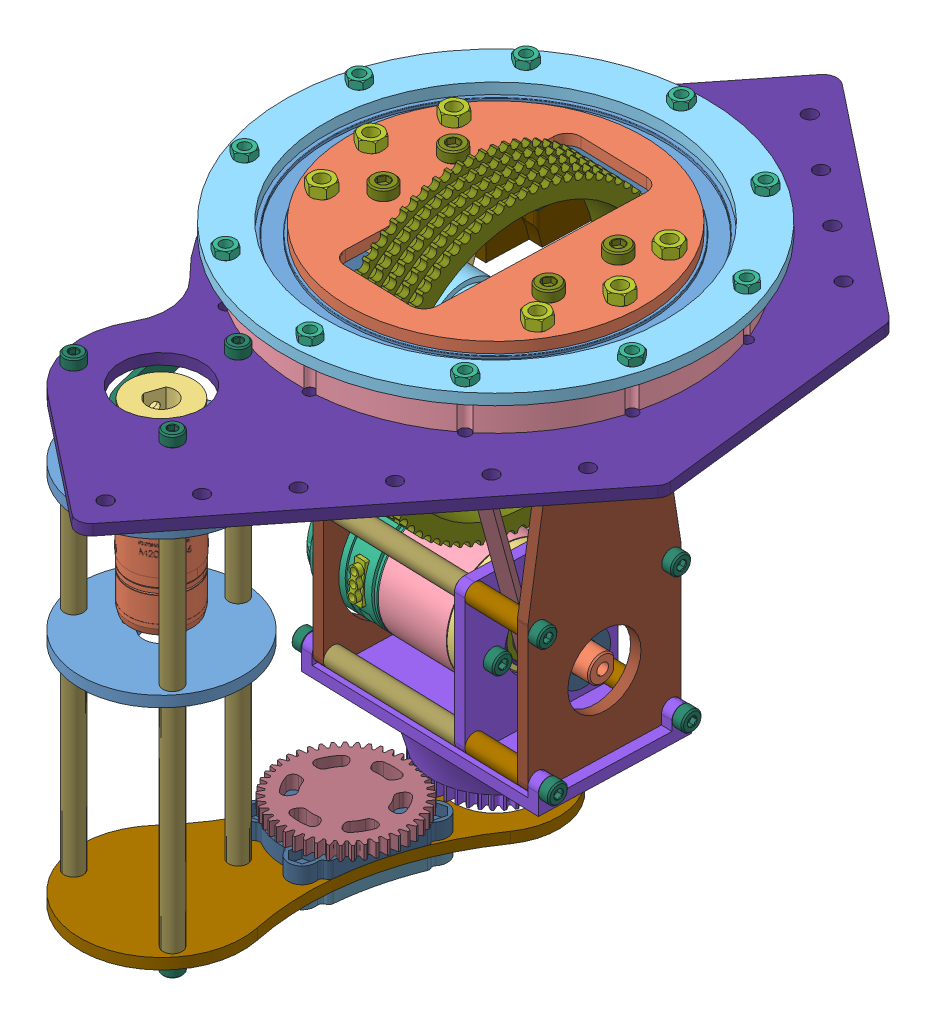
SolidWorks assembly 舵轮装配, configuration 默认. Lengths in mm. (continued)
Mates (geometry in assembly coordinates): (continued)
- 同心68: concentric aligned: cylinder of M3508电机安装延长-1 through (8.8031 -96.0384 93.3761) axis (-0.999547 0 -0.03008) radius 2.1; cylinder of M4螺丝头-14 through (12.8013 -96.0384 93.4965) axis (-0.999547 0 -0.03008) radius 3.6
- 同心69: concentric aligned: cylinder of M3508电机安装延长-1 through (9.3295 -113.5384 75.8841) axis (-0.999547 0 -0.03008) radius 2.1; cylinder of M4螺丝头-13 through (13.3277 -113.5384 76.0044) axis (-0.999547 0 -0.03008) radius 3.6
- 重合43: coincident anti-aligned: plane of M3508电机安装延长-1 through (8.8031 -113.5384 93.3761) normal (0.999547 0 0.03008); plane of M4螺丝头-11 through (8.2767 -113.5384 110.8682) normal (-0.999547 0 -0.03008)
- 重合44: coincident aligned: plane of M4螺丝头-11 through (12.2749 -113.5384 110.9885) normal (0.999547 0 0.03008); plane of M4螺丝头-14 through (12.8013 -96.0384 93.4965) normal (0.999547 0 0.03008)
- 重合45: coincident aligned: plane of M4螺丝头-12 through (12.8013 -131.0384 93.4965) normal (0.999547 0 0.03008); circle of M4螺丝头-13
- 重合46: coincident aligned: plane of M4螺丝头-11 through (12.2749 -113.5384 110.9885) normal (0.999547 0 0.03008); plane of M4螺丝头-12 through (12.8013 -131.0384 93.4965) normal (0.999547 0 0.03008)
- 同心70: concentric anti-aligned: cylinder of M3508电机安装板B-1 through (-45.4733 -15.0564 101.7473) axis (-0.999547 0 -0.03008) radius 2.6; cylinder of M5螺丝头-3 through (-54.4692 -15.0564 101.4766) axis (0.999547 0 0.03008) radius 4.35
- 同心71: concentric anti-aligned: cylinder of M3508电机安装板B-1 through (-44.8717 -15.0564 81.7563) axis (-0.999547 0 -0.03008) radius 2.6; cylinder of M5螺丝头-4 through (-53.8676 -15.0564 81.4856) axis (0.999547 0 0.03008) radius 4.35
- 重合47: coincident anti-aligned: plane of M3508电机安装板B-1 through (-49.1707 -7.5564 91.6315) normal (-0.999547 0 -0.03008); circle of M5螺丝头-4
- 重合48: coincident anti-aligned: plane of M3508电机安装板B-1 through (-49.1707 -7.5564 91.6315) normal (-0.999547 0 -0.03008); plane of M5螺丝头-3 through (-49.4715 -15.0564 101.627) normal (0.999547 0 0.03008)
- 同心72: concentric anti-aligned: cylinder of M3508电机安装板B-1 through (-45.3229 -0.0564 96.7496) axis (-0.999547 0 -0.03008) radius 2.6; cylinder of M5螺丝头-2 through (-54.3188 -0.0564 96.4788) axis (0.999547 0 0.03008) radius 4.35
- 重合49: coincident anti-aligned: plane of M3508电机安装板B-1 through (-49.1707 -7.5564 91.6315) normal (-0.999547 0 -0.03008); plane of M5螺丝头-2 through (-49.3211 -0.0564 96.6292) normal (0.999547 0 0.03008)
- 重合50: coincident anti-aligned: plane of M3508电机安装板B-1 through (-49.1707 -7.5564 91.6315) normal (-0.999547 0 -0.03008); plane of M5螺丝头-1 through (-49.0203 -0.0564 86.6338) normal (0.999547 0 0.03008)
- 同心73: concentric anti-aligned: cylinder of M3508电机安装板B-1 through (-45.0221 -0.0564 86.7541) axis (-0.999547 0 -0.03008) radius 2.6; cylinder of M5螺丝头-1 through (-54.018 -0.0564 86.4834) axis (0.999547 0 0.03008) radius 4.35
- 同心78: concentric aligned: cylinder of HRB 61821薄圈轴承-1 through (-8.689 4.9436 92.8497) axis (0 -1 0) radius 65; cylinder of 舵轮直角安装架-1 through (-8.689 -8.0564 92.8497) axis (0 -1 0) radius 63
- 重合56: coincident anti-aligned: plane of 舵轮上底板-1 through (-8.689 -12.0564 92.8497) normal (0 -1 0); plane of 舵轮转向同步轮 75齿-3 through (-8.6606 -12.0564 92.6837) normal (0 1 0)
- 同心92: concentric aligned: cylinder of 舵轮上底板-1 through (31.7142 -2.0564 117.8264) axis (0 -1 0) radius 2.6; cylinder of 舵轮轴承契合垫B-1 through (31.7142 4.9436 117.8264) axis (0 -1 0) radius 2.6
- 同心93: concentric aligned: cylinder of 舵轮上底板-1 through (31.7142 -2.0564 117.8264) axis (0 -1 0) radius 2.6; cylinder of 舵轮转向同步轮 75齿-3 through (31.7142 23.4436 117.8264) axis (0 -1 0) radius 2.6
- 同心94: concentric aligned: cylinder of 舵轮上底板-1 through (-49.0922 -2.0564 67.8731) axis (0 -1 0) radius 2.6; cylinder of 舵轮转向同步轮 75齿-3 through (-49.0922 23.4436 67.8731) axis (0 -1 0) radius 2.6
- 同心95: concentric aligned: cylinder of 舵轮直角安装架-1 through (-15.1983 -18.0564 205.8519) axis (0 1 0) radius 2.1; cylinder of 舵轮转向电机安装件-1 through (-15.1983 -36.0564 205.8519) axis (0 1 0) radius 2.1
- 同心98: concentric aligned: cylinder of 舵轮直角安装架-1 through (-15.1983 -18.0564 205.8519) axis (0 1 0) radius 2.1; cylinder of 舵轮转向电机安装件-1 through (-15.1983 -36.0564 205.8519) axis (0 1 0) radius 2.1
- 同心99: concentric aligned: cylinder of 舵轮直角安装架-1 through (-58.0411 -18.0564 199.5679) axis (0 1 0) radius 2.1; cylinder of 舵轮转向电机安装件-1 through (-58.0411 -36.0564 199.5679) axis (0 1 0) radius 2.1
- 同心100: concentric aligned: cylinder of 舵轮转向电机安装件-1 through (-33.427 -49.0564 180.9428) axis (0 1 0) radius 1.6; cylinder of RoboMaster M2006 P36直流无刷减速电机.step-2 through (-33.427 -36.0564 180.9428) axis (0 1 0) radius 1.25
- 重合57: coincident anti-aligned: plane of 舵轮转向电机安装件-1 through (-34.8056 -36.0564 190.3422) normal (0 -1 0); plane of RoboMaster M2006 P36直流无刷减速电机.step-2 through (-25.2372 -36.0564 197.911) normal (0 1 0)
- 同心101: concentric aligned: cylinder of 舵轮转向电机安装件-1 through (-34.8056 -49.0564 190.3422) axis (0 1 0) radius 6.6; cylinder of RoboMaster M2006 P36直流无刷减速电机.step-2 through (-34.8056 -19.0564 190.3422) axis (0 1 0) radius 3
- 同心102: concentric anti-aligned: cylinder of 舵轮直角安装架-1 through (-58.0411 -18.0564 199.5679) axis (0 1 0) radius 2.1; cylinder of 螺纹M4_长度20铝柱-5 through (-58.0411 -12.0564 199.5679) axis (0 -1 0) radius 3.5
- 同心103: concentric anti-aligned: cylinder of 舵轮直角安装架-1 through (-31.1775 -18.0564 165.6069) axis (0 1 0) radius 2.1; cylinder of 螺纹M4_长度20铝柱-7 through (-31.1775 -12.0564 165.6069) axis (0 -1 0) radius 3.5
- 同心104: concentric anti-aligned: cylinder of 舵轮直角安装架-1 through (-15.1983 -18.0564 205.8519) axis (0 1 0) radius 2.1; cylinder of 螺纹M4_长度20铝柱-6 through (-15.1983 -12.0564 205.8519) axis (0 -1 0) radius 3.5
- 重合58: coincident anti-aligned: plane of 舵轮转向电机安装件-1 through (-34.8056 -32.0564 190.3422) normal (0 1 0); plane of 螺纹M4_长度20铝柱-6 through (-15.1983 -32.0564 205.8519) normal (0 -1 0)
- 重合59: coincident anti-aligned: plane of 舵轮转向电机安装件-1 through (-34.8056 -32.0564 190.3422) normal (0 1 0); plane of 螺纹M4_长度20铝柱-5 through (-58.0411 -32.0564 199.5679) normal (0 -1 0)
- 重合60: coincident anti-aligned: plane of 舵轮转向电机安装件-1 through (-34.8056 -32.0564 190.3422) normal (0 1 0); plane of 螺纹M4_长度20铝柱-7 through (-31.1775 -32.0564 165.6069) normal (0 -1 0)
- 重合61: coincident anti-aligned: plane of 舵轮直角安装架-1 through (-8.689 -12.0564 92.8497) normal (0 -1 0); plane of 螺纹M4_长度20铝柱-5 through (-58.0411 -12.0564 199.5679) normal (0 1 0)
- 同心105: concentric anti-aligned: cylinder of RoboMaster M2006 P36直流无刷减速电机.step-2 through (-34.8056 -19.0564 190.3422) axis (0 1 0) radius 3; cylinder of 舵轮转向驱动同步轮15齿-1 through (-34.8056 -7.5564 190.3422) axis (0 -1 0) radius 5.15
- 重合62: coincident aligned: plane of 舵轮转向同步轮 75齿-3 through (-8.6606 -12.0564 92.6837) normal (0 1 0); plane of 舵轮转向驱动同步轮15齿-1 through (-34.8056 -12.0564 190.3422) normal (0 1 0)
- 重合63: coincident anti-aligned: plane of HRB 61821薄圈轴承-1 through (-8.689 -8.0564 92.8497) normal (0 -1 0); plane of 舵轮直角安装架-1 through (-8.689 -8.0564 92.8497) normal (0 1 0)
- 同心106: concentric anti-aligned: cylinder of 舵轮转向同步轮 75齿-3 through (31.7142 -19.5564 117.8264) axis (0 -1 0) radius 4.5; cylinder of M5螺丝头-10 through (31.7142 -24.5564 117.8264) axis (0 1 0) radius 4.35
- 同心107: concentric aligned: cylinder of M3508电机安装板-1 through (32.4914 -15.0564 104.0935) axis (-0.999547 0 -0.03008) radius 2.6; cylinder of M5螺丝头-12 through (37.4891 -15.0564 104.2439) axis (-0.999547 0 -0.03008) radius 4.35
- 重合64: coincident anti-aligned: plane of M3508电机安装板-1 through (32.7922 -7.5564 94.0981) normal (0.999547 0 0.03008); plane of M5螺丝头-12 through (32.4914 -15.0564 104.0935) normal (-0.999547 0 -0.03008)
- 重合65: coincident anti-aligned: plane of 舵轮转向同步轮 75齿-3 through (38.7895 -19.5564 94.2785) normal (0 -1 0); plane of M5螺丝头-11 through (38.7895 -19.5564 94.2785) normal (0 1 0)
- 同心108: concentric aligned: cylinder of 舵轮转向同步轮 75齿-3 through (38.7895 -19.5564 94.2785) axis (0 -1 0) radius 4.5; circle of M5螺丝头-11
- 同心109: concentric anti-aligned: cylinder of 舵轮转向同步轮 75齿-3 through (33.143 -19.5564 70.3479) axis (0 -1 0) radius 4.5; cylinder of M5螺丝头-13 through (33.143 -24.5564 70.3479) axis (0 1 0) radius 4.35
- 重合66: coincident anti-aligned: plane of 舵轮转向同步轮 75齿-3 through (33.143 -19.5564 70.3479) normal (0 -1 0); plane of M5螺丝头-13 through (33.143 -19.5564 70.3479) normal (0 1 0)
- 同心110: concentric aligned: cylinder of M3508电机安装板-1 through (33.093 -15.0564 84.1026) axis (-0.999547 0 -0.03008) radius 2.6; cylinder of M5螺丝头-14 through (38.0907 -15.0564 84.253) axis (-0.999547 0 -0.03008) radius 4.35
- 重合67: coincident anti-aligned: plane of M3508电机安装板-1 through (32.7922 -7.5564 94.0981) normal (0.999547 0 0.03008); plane of M5螺丝头-14 through (33.093 -15.0564 84.1026) normal (-0.999547 0 -0.03008)
- 重合68: coincident anti-aligned: plane of 舵轮转向同步轮 75齿-3 through (31.7142 -19.5564 117.8264) normal (0 -1 0); plane of M5螺丝头-10 through (31.7142 -19.5564 117.8264) normal (0 1 0)
- 同心111: concentric anti-aligned: cylinder of 舵轮转向同步轮 75齿-3 through (-50.521 -19.5564 115.3516) axis (0 -1 0) radius 4.5; cylinder of M5螺丝头-7 through (-50.521 -24.5564 115.3516) axis (0 1 0) radius 4.35
- 同心112: concentric anti-aligned: cylinder of 舵轮转向同步轮 75齿-3 through (-56.1675 -19.5564 91.4209) axis (0 -1 0) radius 4.5; cylinder of M5螺丝头-8 through (-56.1675 -24.5564 91.4209) axis (0 1 0) radius 4.35
- 同心113: concentric anti-aligned: cylinder of 舵轮转向同步轮 75齿-3 through (-49.0922 -19.5564 67.8731) axis (0 -1 0) radius 4.5; cylinder of M5螺丝头-9 through (-49.0922 -24.5564 67.8731) axis (0 1 0) radius 4.35
- 重合69: coincident anti-aligned: plane of 舵轮转向同步轮 75齿-3 through (-49.0922 -19.5564 67.8731) normal (0 -1 0); plane of M5螺丝头-9 through (-49.0922 -19.5564 67.8731) normal (0 1 0)
- 重合70: coincident anti-aligned: plane of 舵轮转向同步轮 75齿-3 through (-56.1675 -19.5564 91.4209) normal (0 -1 0); plane of M5螺丝头-8 through (-56.1675 -19.5564 91.4209) normal (0 1 0)
- 重合71: coincident anti-aligned: plane of 舵轮转向同步轮 75齿-3 through (-50.521 -19.5564 115.3516) normal (0 -1 0); plane of M5螺丝头-7 through (-50.521 -19.5564 115.3516) normal (0 1 0)
- 同心114: concentric aligned: cylinder of HRB 61821薄圈轴承-1 through (-8.689 4.9436 92.8497) axis (0 -1 0) radius 65; cylinder of 舵轮大轴承定位环-1 through (-8.689 4.9436 92.8497) axis (0 -1 0) radius 72.1
- 重合72: coincident anti-aligned: plane of 舵轮直角安装架-1 through (-8.689 -8.0564 92.8497) normal (0 1 0); plane of 舵轮大轴承定位环-1 through (-8.689 -8.0564 92.8497) normal (0 -1 0)
- 同心115: concentric aligned: cylinder of 舵轮直角安装架-1 through (-76.1543 -18.0564 118.2829) axis (0 1 0) radius 2.05; cylinder of 舵轮大轴承定位环-1 through (-76.1543 -8.0564 118.2829) axis (0 1 0) radius 2.1
- 同心116: concentric aligned: cylinder of 舵轮大轴承定位环-1 through (60.8408 -8.0564 111.9289) axis (0 1 0) radius 2.1; cylinder of 轴承压住-1 through (60.8408 4.9436 111.9289) axis (0 1 0) radius 2.05
- 同心118: concentric aligned: cylinder of 舵轮大轴承定位环-1 through (36.3473 -8.0564 149.1537) axis (0 1 0) radius 2.1; circle of 轴承压住-1
- 重合77: coincident anti-aligned: plane of 舵轮大轴承定位环-1 through (-8.689 4.9436 92.8497) normal (0 1 0); plane of 轴承压住-1 through (-8.689 4.9436 92.8497) normal (0 -1 0)
- 同心121: concentric aligned: cylinder of 舵轮直角安装架-1 through (58.7762 -18.0564 67.4165) axis (0 1 0) radius 2.05; cylinder of M4螺丝头-18 through (58.7762 -16.0564 67.4165) axis (0 1 0) radius 3.6
- 同心122: concentric aligned: cylinder of 舵轮直角安装架-1 through (60.8408 -18.0564 111.9289) axis (0 1 0) radius 2.05; cylinder of M4螺丝头-19 through (60.8408 -16.0564 111.9289) axis (0 1 0) radius 3.6
- 同心123: concentric aligned: cylinder of 舵轮直角安装架-1 through (36.3473 -18.0564 149.1537) axis (0 1 0) radius 2.05; cylinder of M4螺丝头-20 through (36.3473 -16.0564 149.1537) axis (0 1 0) radius 3.6
- 同心124: concentric aligned: cylinder of 舵轮直角安装架-1 through (-5.3485 -18.0564 164.8723) axis (0 1 0) radius 2.05; cylinder of M4螺丝头-21 through (-5.3485 -16.0564 164.8723) axis (0 1 0) radius 3.6
- 同心125: concentric aligned: cylinder of 舵轮直角安装架-1 through (-48.3203 -18.0564 153.0807) axis (0 1 0) radius 2.05; cylinder of M4螺丝头-22 through (-48.3203 -16.0564 153.0807) axis (0 1 0) radius 3.6
- 同心126: concentric aligned: cylinder of 舵轮直角安装架-1 through (-76.1543 -18.0564 118.2829) axis (0 1 0) radius 2.05; cylinder of M4螺丝头-23 through (-76.1543 -16.0564 118.2829) axis (0 1 0) radius 3.6
- 同心127: concentric aligned: cylinder of 舵轮直角安装架-1 through (-78.2188 -18.0564 73.7705) axis (0 1 0) radius 2.05; cylinder of M4螺丝头-24 through (-78.2188 -16.0564 73.7705) axis (0 1 0) radius 3.6
- 同心128: concentric aligned: cylinder of 舵轮直角安装架-1 through (-53.7253 -18.0564 36.5458) axis (0 1 0) radius 2.05; cylinder of M4螺丝头-15 through (-53.7253 -16.0564 36.5458) axis (0 1 0) radius 3.6
- 同心129: concentric aligned: cylinder of 舵轮直角安装架-1 through (-12.0295 -18.0564 20.8272) axis (0 1 0) radius 2.05; cylinder of M4螺丝头-16 through (-12.0295 -16.0564 20.8272) axis (0 1 0) radius 3.6
- 同心130: concentric aligned: cylinder of 舵轮直角安装架-1 through (30.9423 -18.0564 32.6188) axis (0 1 0) radius 2.05; cylinder of M4螺丝头-17 through (30.9423 -16.0564 32.6188) axis (0 1 0) radius 3.6
- 重合79: coincident anti-aligned: plane of 舵轮直角安装架-1 through (-8.689 -12.0564 92.8497) normal (0 -1 0); plane of M4螺丝头-18 through (58.7762 -12.0564 67.4165) normal (0 1 0)
- 重合80: coincident aligned: plane of M4螺丝头-17 through (30.9423 -16.0564 32.6188) normal (0 -1 0); plane of M4螺丝头-18 through (58.7762 -16.0564 67.4165) normal (0 -1 0)
- 重合81: coincident aligned: plane of M4螺丝头-16 through (-12.0295 -16.0564 20.8272) normal (0 -1 0); plane of M4螺丝头-17 through (30.9423 -16.0564 32.6188) normal (0 -1 0)
- 重合82: coincident aligned: plane of M4螺丝头-15 through (-53.7253 -16.0564 36.5458) normal (0 -1 0); plane of M4螺丝头-16 through (-12.0295 -16.0564 20.8272) normal (0 -1 0)
- 重合83: coincident aligned: plane of M4螺丝头-15 through (-53.7253 -16.0564 36.5458) normal (0 -1 0); plane of M4螺丝头-24 through (-78.2188 -16.0564 73.7705) normal (0 -1 0)
- 重合84: coincident aligned: plane of M4螺丝头-23 through (-76.1543 -16.0564 118.2829) normal (0 -1 0); plane of M4螺丝头-24 through (-78.2188 -16.0564 73.7705) normal (0 -1 0)
- 重合85: coincident aligned: plane of M4螺丝头-22 through (-48.3203 -16.0564 153.0807) normal (0 -1 0); plane of M4螺丝头-23 through (-76.1543 -16.0564 118.2829) normal (0 -1 0)
- 重合86: coincident aligned: plane of M4螺丝头-21 through (-5.3485 -16.0564 164.8723) normal (0 -1 0); plane of M4螺丝头-22 through (-48.3203 -16.0564 153.0807) normal (0 -1 0)
- 重合87: coincident aligned: plane of M4螺丝头-20 through (36.3473 -16.0564 149.1537) normal (0 -1 0); plane of M4螺丝头-21 through (-5.3485 -16.0564 164.8723) normal (0 -1 0)
- 重合88: coincident aligned: plane of M4螺丝头-19 through (60.8408 -16.0564 111.9289) normal (0 -1 0); plane of M4螺丝头-20 through (36.3473 -16.0564 149.1537) normal (0 -1 0)
- 同心131: concentric anti-aligned: cylinder of 轴承压住-1 through (58.7762 4.9436 67.4165) axis (0 1 0) radius 2.05; cylinder of M4螺母-10 through (58.7762 11.9436 67.4165) axis (0 -1 0) radius 2
- 同心132: concentric anti-aligned: cylinder of 轴承压住-1 through (60.8408 4.9436 111.9289) axis (0 1 0) radius 2.05; cylinder of M4螺母-1 through (60.8408 11.9436 111.9289) axis (0 -1 0) radius 2
- 同心133: concentric anti-aligned: cylinder of 轴承压住-1 through (36.3473 4.9436 149.1537) axis (0 1 0) radius 2.05; cylinder of M4螺母-11 through (36.3473 11.9436 149.1537) axis (0 -1 0) radius 2
- 同心134: concentric anti-aligned: cylinder of 轴承压住-1 through (-5.3485 4.9436 164.8723) axis (0 1 0) radius 2.05; cylinder of M4螺母-3 through (-5.3485 11.9436 164.8723) axis (0 -1 0) radius 2
- 同心135: concentric anti-aligned: cylinder of 轴承压住-1 through (-48.3203 4.9436 153.0807) axis (0 1 0) radius 2.05; cylinder of M4螺母-4 through (-48.3203 11.9436 153.0807) axis (0 -1 0) radius 2
- 同心136: concentric anti-aligned: cylinder of 轴承压住-1 through (-76.1543 4.9436 118.2829) axis (0 1 0) radius 2.05; cylinder of M4螺母-5 through (-76.1543 11.9436 118.2829) axis (0 -1 0) radius 2
- 同心137: concentric anti-aligned: cylinder of 轴承压住-1 through (-78.2188 4.9436 73.7705) axis (0 1 0) radius 2.05; cylinder of M4螺母-6 through (-78.2188 11.9436 73.7705) axis (0 -1 0) radius 2
- 同心138: concentric anti-aligned: cylinder of 轴承压住-1 through (-53.7253 4.9436 36.5458) axis (0 1 0) radius 2.05; cylinder of M4螺母-7 through (-53.7253 11.9436 36.5458) axis (0 -1 0) radius 2
- 同心139: concentric anti-aligned: cylinder of 轴承压住-1 through (30.9423 4.9436 32.6188) axis (0 1 0) radius 2.05; cylinder of M4螺母-9 through (30.9423 11.9436 32.6188) axis (0 -1 0) radius 2
- 同心140: concentric anti-aligned: cylinder of 轴承压住-1 through (-12.0295 4.9436 20.8272) axis (0 1 0) radius 2.05; cylinder of M4螺母-8 through (-12.0295 11.9436 20.8272) axis (0 -1 0) radius 2
- 重合89: coincident anti-aligned: plane of 轴承压住-1 through (-8.689 8.9436 92.8497) normal (0 1 0); plane of M4螺母-10 through (58.7762 8.9436 67.4165) normal (0 -1 0)
- 重合90: coincident aligned: plane of M4螺母-9 through (30.9423 11.9436 32.6188) normal (0 1 0); plane of M4螺母-10 through (58.7762 11.9436 67.4165) normal (0 1 0)
- 重合91: coincident aligned: plane of M4螺母-8 through (-12.0295 11.9436 20.8272) normal (0 1 0); plane of M4螺母-9 through (30.9423 11.9436 32.6188) normal (0 1 0)
- 重合92: coincident aligned: plane of M4螺母-7 through (-53.7253 11.9436 36.5458) normal (0 1 0); plane of M4螺母-8 through (-12.0295 11.9436 20.8272) normal (0 1 0)
- 重合93: coincident aligned: plane of M4螺母-6 through (-78.2188 11.9436 73.7705) normal (0 1 0); plane of M4螺母-7 through (-53.7253 11.9436 36.5458) normal (0 1 0)
- 重合94: coincident aligned: plane of M4螺母-5 through (-76.1543 11.9436 118.2829) normal (0 1 0); plane of M4螺母-6 through (-78.2188 11.9436 73.7705) normal (0 1 0)
- 重合95: coincident aligned: plane of M4螺母-4 through (-48.3203 11.9436 153.0807) normal (0 1 0); plane of M4螺母-5 through (-76.1543 11.9436 118.2829) normal (0 1 0)
- 重合96: coincident aligned: plane of M4螺母-3 through (-5.3485 11.9436 164.8723) normal (0 1 0); plane of M4螺母-4 through (-48.3203 11.9436 153.0807) normal (0 1 0)
- 重合97: coincident aligned: plane of M4螺母-3 through (-5.3485 11.9436 164.8723) normal (0 1 0); plane of M4螺母-11 through (36.3473 11.9436 149.1537) normal (0 1 0)
- 重合98: coincident aligned: plane of M4螺母-1 through (60.8408 11.9436 111.9289) normal (0 1 0); plane of M4螺母-11 through (36.3473 11.9436 149.1537) normal (0 1 0)
- 同心141: concentric aligned: cylinder of 舵轮底板-1 through (-38.5517 14.9436 104.4567) axis (0 -1 0) radius 2.6; cylinder of M5螺丝头-18 through (-38.5517 13.9436 104.4567) axis (0 -1 0) radius 4.35
- 同心142: concentric aligned: cylinder of 舵轮底板-1 through (-37.7997 14.9436 79.468) axis (0 -1 0) radius 2.6; cylinder of M5螺丝头-17 through (-37.7997 13.9436 79.468) axis (0 -1 0) radius 4.35
- 同心143: concentric aligned: cylinder of 舵轮底板-1 through (24.4198 104.9436 106.3518) axis (0 -1 0) radius 2.6; cylinder of M5螺丝头-15 through (24.4198 13.9436 106.3518) axis (0 -1 0) radius 4.35
- 同心144: concentric aligned: cylinder of 舵轮底板-1 through (25.1718 104.9436 81.3631) axis (0 -1 0) radius 2.6; cylinder of M5螺丝头-16 through (25.1718 13.9436 81.3631) axis (0 -1 0) radius 4.35
- 重合99: coincident anti-aligned: plane of 舵轮底板-1 through (-8.689 8.9436 92.8497) normal (0 1 0); circle of M5螺丝头-16
- 重合100: coincident aligned: plane of M5螺丝头-15 through (24.4198 13.9436 106.3518) normal (0 1 0); plane of M5螺丝头-16 through (25.1718 13.9436 81.3631) normal (0 1 0)
- 重合101: coincident aligned: plane of M5螺丝头-16 through (25.1718 13.9436 81.3631) normal (0 1 0); plane of M5螺丝头-17 through (-37.7997 13.9436 79.468) normal (0 1 0)
- 重合102: coincident aligned: plane of M5螺丝头-17 through (-37.7997 13.9436 79.468) normal (0 1 0); plane of M5螺丝头-18 through (-38.5517 13.9436 104.4567) normal (0 1 0)
- 同心145: concentric aligned: cylinder of 螺纹M4_长度20铝柱-5 through (-58.0411 -12.0564 199.5679) axis (0 -1 0) radius 3.5; cylinder of M4螺丝头-26 through (-58.0411 -4.0564 199.5679) axis (0 -1 0) radius 3.6
- 同心146: concentric aligned: cylinder of 螺纹M4_长度20铝柱-6 through (-15.1983 -12.0564 205.8519) axis (0 -1 0) radius 3.5; cylinder of M4螺丝头-25 through (-15.1983 -4.0564 205.8519) axis (0 -1 0) radius 3.6
- 同心147: concentric anti-aligned: cylinder of 舵轮直角安装架-1 through (-31.1775 -18.0564 165.6069) axis (0 1 0) radius 2.1; cylinder of M4螺丝头-27 through (-31.1775 -4.0564 165.6069) axis (0 -1 0) radius 3.6
- 重合103: coincident anti-aligned: plane of 舵轮直角安装架-1 through (-8.689 -8.0564 92.8497) normal (0 1 0); plane of M4螺丝头-27 through (-31.1775 -8.0564 165.6069) normal (0 -1 0)
- 重合104: coincident aligned: plane of M4螺丝头-26 through (-58.0411 -4.0564 199.5679) normal (0 1 0); plane of M4螺丝头-27 through (-31.1775 -4.0564 165.6069) normal (0 1 0)
- 重合105: coincident aligned: plane of M4螺丝头-25 through (-15.1983 -4.0564 205.8519) normal (0 1 0); plane of M4螺丝头-26 through (-58.0411 -4.0564 199.5679) normal (0 1 0)
- 同心151: concentric aligned: cylinder of 舵轮底板-1 through (-49.0922 14.9436 67.8731) axis (0 -1 0) radius 2.6; cylinder of M5螺母-1 through (-49.0922 12.9436 67.8731) axis (0 -1 0) radius 2.5
- 同心152: concentric aligned: cylinder of 舵轮底板-1 through (-56.1675 14.9436 91.4209) axis (0 -1 0) radius 2.6; cylinder of M5螺母-2 through (-56.1675 12.9436 91.4209) axis (0 -1 0) radius 2.5
- 同心153: concentric aligned: cylinder of 舵轮底板-1 through (-50.521 14.9436 115.3516) axis (0 -1 0) radius 2.6; cylinder of M5螺母-3 through (-50.521 12.9436 115.3516) axis (0 -1 0) radius 2.5
- 同心154: concentric aligned: cylinder of 舵轮底板-1 through (31.7142 14.9436 117.8264) axis (0 -1 0) radius 2.6; cylinder of M5螺母-4 through (31.7142 12.9436 117.8264) axis (0 -1 0) radius 2.5
- 同心155: concentric aligned: cylinder of 舵轮底板-1 through (38.7895 14.9436 94.2785) axis (0 -1 0) radius 2.6; cylinder of M5螺母-5 through (38.7895 12.9436 94.2785) axis (0 -1 0) radius 2.5
- 同心156: concentric aligned: cylinder of 舵轮底板-1 through (33.143 14.9436 70.3479) axis (0 -1 0) radius 2.6; cylinder of M5螺母-6 through (33.143 12.9436 70.3479) axis (0 -1 0) radius 2.5
- 重合109: coincident anti-aligned: plane of 舵轮底板-1 through (-8.689 8.9436 92.8497) normal (0 1 0); plane of M5螺母-6 through (33.143 8.9436 70.3479) normal (0 -1 0)
- 重合110: coincident aligned: plane of M5螺母-5 through (38.7895 12.9436 94.2785) normal (0 1 0); plane of M5螺母-6 through (33.143 12.9436 70.3479) normal (0 1 0)
- 重合111: coincident aligned: plane of M5螺母-4 through (31.7142 12.9436 117.8264) normal (0 1 0); plane of M5螺母-6 through (33.143 12.9436 70.3479) normal (0 1 0)
- 重合112: coincident aligned: plane of M5螺母-3 through (-50.521 12.9436 115.3516) normal (0 1 0); plane of M5螺母-4 through (31.7142 12.9436 117.8264) normal (0 1 0)
- 重合113: coincident aligned: plane of M5螺母-2 through (-56.1675 12.9436 91.4209) normal (0 1 0); plane of M5螺母-3 through (-50.521 12.9436 115.3516) normal (0 1 0)
- 重合114: coincident aligned: plane of M5螺母-1 through (-49.0922 12.9436 67.8731) normal (0 1 0); plane of M5螺母-2 through (-56.1675 12.9436 91.4209) normal (0 1 0)
- 同心157: concentric anti-aligned: cylinder of 舵轮转向电机安装件-1 through (-15.1983 -36.0564 205.8519) axis (0 1 0) radius 2.1; cylinder of 螺纹M4_长度50铝柱-6 through (-15.1983 -36.0564 205.8519) axis (0 -1 0) radius 3.5
- 同心158: concentric anti-aligned: cylinder of 舵轮转向电机安装件-1 through (-58.0411 -36.0564 199.5679) axis (0 1 0) radius 2.1; cylinder of 螺纹M4_长度50铝柱-5 through (-58.0411 -36.0564 199.5679) axis (0 -1 0) radius 3.5
- 同心159: concentric anti-aligned: cylinder of 舵轮转向电机安装件-1 through (-31.1775 -36.0564 165.6069) axis (0 1 0) radius 2.1; cylinder of 螺纹M4_长度50铝柱-7 through (-31.1775 -36.0564 165.6069) axis (0 -1 0) radius 3.5
- 重合115: coincident anti-aligned: plane of 舵轮转向电机安装件-1 through (-34.8056 -36.0564 190.3422) normal (0 -1 0); plane of 螺纹M4_长度50铝柱-7 through (-31.1775 -36.0564 165.6069) normal (0 1 0)
- 重合116: coincident anti-aligned: plane of 舵轮转向电机安装件-1 through (-34.8056 -36.0564 190.3422) normal (0 -1 0); plane of 螺纹M4_长度50铝柱-5 through (-58.0411 -36.0564 199.5679) normal (0 1 0)
- 重合117: coincident anti-aligned: plane of 舵轮转向电机安装件-1 through (-34.8056 -36.0564 190.3422) normal (0 -1 0); plane of 螺纹M4_长度50铝柱-6 through (-15.1983 -36.0564 205.8519) normal (0 1 0)
- 同心160: concentric anti-aligned: cylinder of 螺纹M4_长度50铝柱-6 through (-15.1983 -36.0564 205.8519) axis (0 -1 0) radius 2; cylinder of 舵轮转向电机安装件-2 through (-15.1983 -90.0564 205.8519) axis (0 1 0) radius 2.1
- 同心161: concentric anti-aligned: cylinder of 螺纹M4_长度50铝柱-7 through (-31.1775 -36.0564 165.6069) axis (0 -1 0) radius 2; cylinder of 舵轮转向电机安装件-2 through (-31.1775 -90.0564 165.6069) axis (0 1 0) radius 2.1
- 重合118: coincident anti-aligned: plane of 螺纹M4_长度50铝柱-6 through (-15.1983 -86.0564 205.8519) normal (0 -1 0); plane of 舵轮转向电机安装件-2 through (-34.8056 -86.0564 190.3422) normal (0 1 0)
- 同心168: concentric anti-aligned: cylinder of M3508电机安装板-1 through (22.0748 -137.5384 117.7864) axis (0.999547 0 0.03008) radius 2.1; cylinder of 舵轮线引导和角度定位3D打印件-1 through (36.0685 -137.5384 118.2075) axis (-0.999547 0 -0.03008) radius 2.1
- 同心169: concentric anti-aligned: cylinder of M3508电机安装板-1 through (23.5186 -137.5384 69.8081) axis (0.999547 0 0.03008) radius 2.1; cylinder of 舵轮线引导和角度定位3D打印件-1 through (37.5123 -137.5384 70.2292) axis (-0.999547 0 -0.03008) radius 2.1
- 重合125: coincident anti-aligned: plane of M3508电机安装板-1 through (32.7922 -7.5564 94.0981) normal (0.999547 0 0.03008); plane of 舵轮线引导和角度定位3D打印件-1 through (32.7922 -141.0384 94.0981) normal (-0.999547 0 -0.03008)
- 重合129: coincident anti-aligned: plane of 舵轮线引导和角度定位3D打印件-1 through (-8.3392 -145.0384 92.8603) normal (0 -1 0); plane of C620无刷电机调速器.STEP-1/7.STEP-1 through (-28.3301 -145.0384 92.2587) normal (0 1 0)
- 同心173: concentric aligned: circle of C620无刷电机调速器.STEP-1/7.STEP-1; cylinder of 舵轮线引导和角度定位3D打印件-1 through (-51.1906 -135.0384 100.5748) axis (0 -1 0) radius 1.1
- 同心174: concentric aligned: cylinder of 舵轮线引导和角度定位3D打印件-1 through (-50.6492 -135.0384 82.5829) axis (0 -1 0) radius 1.1; cylinder of C620无刷电机调速器.STEP-1/7.STEP-1 through (-50.6492 -135.5384 82.5829) axis (0 -1 0) radius 1
- 同心175: concentric anti-aligned: cylinder of RoboMaster M3508直流无刷减速电-1/2_ASM-1/16_1-1 through (4.2785 -113.5384 110.7479) axis (0.999547 0 0.03008) radius 1.65; cylinder of M4螺丝头-11 through (12.2749 -113.5384 110.9885) axis (-0.999547 0 -0.03008) radius 3.6
- 同心183: concentric aligned: cylinder of 理线和舵轮角度定位支撑-1 through (-26.3393 -146.5564 114.2844) axis (0 -1 0) radius 1.65; cylinder of 舵轮角度定位第二齿轮轴承锁定-1 through (-26.3393 -156.0564 114.2844) axis (0 -1 0) radius 1.6
- 同心184: concentric aligned: cylinder of 理线和舵轮角度定位支撑-1 through (-36.6462 -146.5564 152.7652) axis (0 -1 0) radius 1.65; cylinder of 舵轮角度定位第二齿轮轴承锁定-1 through (-36.6462 -156.0564 152.7652) axis (0 -1 0) radius 1.6
- 同心185: concentric anti-aligned: cylinder of 舵轮角度定位第二齿轮轴承锁定-1 through (-20.3843 -170.0564 136.5001) axis (0 1 0) radius 13.6; cylinder of 6704zz轴承-1 through (-20.3843 -166.0564 136.5001) axis (0 -1 0) radius 13.5
- 重合134: coincident anti-aligned: plane of 理线和舵轮角度定位支撑-1 through (-34.8056 -170.0564 190.3422) normal (0 1 0); plane of 6704zz轴承-1 through (-20.3843 -170.0564 136.5001) normal (0 -1 0)
- 同心186: concentric anti-aligned: cylinder of 舵轮转向电机安装件-2 through (-15.1983 -90.0564 205.8519) axis (0 1 0) radius 2.1; cylinder of 螺纹M4_长度80铝柱-1 through (-15.1983 -90.0564 205.8519) axis (0 -1 0) radius 3.5
- 同心187: concentric anti-aligned: cylinder of 舵轮转向电机安装件-2 through (-58.0411 -90.0564 199.5679) axis (0 1 0) radius 2.1; cylinder of 螺纹M4_长度80铝柱-3 through (-58.0411 -90.0564 199.5679) axis (0 -1 0) radius 3.5
- 同心188: concentric anti-aligned: cylinder of 舵轮转向电机安装件-2 through (-31.1775 -90.0564 165.6069) axis (0 1 0) radius 2.1; cylinder of 螺纹M4_长度80铝柱-2 through (-31.1775 -90.0564 165.6069) axis (0 -1 0) radius 3.5
- 重合135: coincident aligned: plane of 螺纹M4_长度80铝柱-1 through (-15.1983 -170.0564 205.8519) normal (0 -1 0); plane of 螺纹M4_长度80铝柱-3 through (-58.0411 -170.0564 199.5679) normal (0 -1 0)
- 重合136: coincident aligned: plane of 螺纹M4_长度80铝柱-2 through (-31.1775 -170.0564 165.6069) normal (0 -1 0); plane of 螺纹M4_长度80铝柱-3 through (-58.0411 -170.0564 199.5679) normal (0 -1 0)
- 重合137: coincident anti-aligned: plane of 舵轮转向电机安装件-2 through (-34.8056 -90.0564 190.3422) normal (0 -1 0); plane of 螺纹M4_长度80铝柱-3 through (-58.0411 -90.0564 199.5679) normal (0 1 0)
- 重合138: coincident anti-aligned: plane of 理线和舵轮角度定位支撑-1 through (-34.8056 -170.0564 190.3422) normal (0 1 0); plane of 螺纹M4_长度80铝柱-1 through (-15.1983 -170.0564 205.8519) normal (0 -1 0)
- 重合139: coincident anti-aligned: plane of 理线和舵轮角度定位支撑-1 through (-34.8056 -170.0564 190.3422) normal (0 1 0); plane of 舵轮角度定位第二齿轮轴承锁定-1 through (-20.3843 -170.0564 136.5001) normal (0 -1 0)
- 同心189: concentric anti-aligned: cylinder of 6704zz轴承-1 through (-20.3843 -166.0564 136.5001) axis (0 -1 0) radius 10; cylinder of 舵轮角度定位第二齿轮-1 through (-20.3843 -167.5564 136.5001) axis (0 1 0) radius 10
- 同心190: concentric anti-aligned: cylinder of 理线和舵轮角度定位支撑-1 through (-58.0411 -174.0564 199.5679) axis (0 1 0) radius 2.1; cylinder of 螺纹M4_长度80铝柱-3 through (-58.0411 -90.0564 199.5679) axis (0 -1 0) radius 3.5
- 同心191: concentric anti-aligned: cylinder of 理线和舵轮角度定位支撑-1 through (-31.1775 -174.0564 165.6069) axis (0 1 0) radius 2.1; cylinder of 螺纹M4_长度80铝柱-2 through (-31.1775 -90.0564 165.6069) axis (0 -1 0) radius 2
- 重合141: coincident anti-aligned: plane of 6704zz轴承-1 through (-20.3843 -166.0564 136.5001) normal (0 1 0); plane of 舵轮角度定位第二齿轮-1 through (-20.3843 -166.0564 136.5001) normal (0 -1 0)
- 同心192: concentric aligned: cylinder of 舵轮线引导和角度定位3D打印件-1 through (-54.1907 -137.5384 115.4913) axis (0.999547 0 0.03008) radius 2.1; cylinder of M4螺丝头-34 through (-58.1889 -137.5384 115.371) axis (0.999547 0 0.03008) radius 3.6
- 同心193: concentric aligned: cylinder of 舵轮线引导和角度定位3D打印件-1 through (-52.7468 -137.5384 67.513) axis (0.999547 0 0.03008) radius 2.1; cylinder of M4螺丝头-31 through (-56.745 -137.5384 67.3927) axis (0.999547 0 0.03008) radius 3.6
- 重合142: coincident aligned: plane of M4螺丝头-31 through (-56.745 -137.5384 67.3927) normal (-0.999547 0 -0.03008); plane of M4螺丝头-34 through (-58.1889 -137.5384 115.371) normal (-0.999547 0 -0.03008)
- 重合143: coincident anti-aligned: plane of 舵轮线引导和角度定位3D打印件-1 through (-53.4687 -141.0384 91.5022) normal (-0.999547 0 -0.03008); plane of M4螺丝头-31 through (-52.7468 -137.5384 67.513) normal (0.999547 0 0.03008)
- 同心194: concentric aligned: cylinder of 舵轮线引导和角度定位3D打印件-1 through (36.0685 -137.5384 118.2075) axis (-0.999547 0 -0.03008) radius 2.1; cylinder of M4螺丝头-32 through (40.0667 -137.5384 118.3278) axis (-0.999547 0 -0.03008) radius 3.6
- 同心195: concentric aligned: cylinder of 舵轮线引导和角度定位3D打印件-1 through (37.5123 -137.5384 70.2292) axis (-0.999547 0 -0.03008) radius 2.1; cylinder of M4螺丝头-33 through (41.5105 -137.5384 70.3496) axis (-0.999547 0 -0.03008) radius 3.6
- 重合144: coincident anti-aligned: plane of 舵轮线引导和角度定位3D打印件-1 through (36.7904 -141.0384 94.2184) normal (0.999547 0 0.03008); plane of M4螺丝头-32 through (36.0685 -137.5384 118.2075) normal (-0.999547 0 -0.03008)
- 重合145: coincident aligned: plane of M4螺丝头-32 through (40.0667 -137.5384 118.3278) normal (0.999547 0 0.03008); plane of M4螺丝头-33 through (41.5105 -137.5384 70.3496) normal (0.999547 0 0.03008)
- 同心196: concentric aligned: cylinder of 理线和舵轮角度定位支撑-1 through (-31.1775 -174.0564 165.6069) axis (0 1 0) radius 2.1; cylinder of M4螺丝头-28 through (-31.1775 -178.0564 165.6069) axis (0 1 0) radius 3.6
- 重合146: coincident anti-aligned: plane of 理线和舵轮角度定位支撑-1 through (-34.8056 -174.0564 190.3422) normal (0 -1 0); plane of M4螺丝头-28 through (-31.1775 -174.0564 165.6069) normal (0 1 0)
- 同心197: concentric aligned: cylinder of 理线和舵轮角度定位支撑-1 through (-15.1983 -174.0564 205.8519) axis (0 1 0) radius 2.1; cylinder of M4螺丝头-30 through (-15.1983 -178.0564 205.8519) axis (0 1 0) radius 3.6
- 重合147: coincident aligned: plane of M4螺丝头-28 through (-31.1775 -178.0564 165.6069) normal (0 -1 0); plane of M4螺丝头-30 through (-15.1983 -178.0564 205.8519) normal (0 -1 0)
- 同心198: concentric aligned: cylinder of 理线和舵轮角度定位支撑-1 through (-58.0411 -174.0564 199.5679) axis (0 1 0) radius 2.1; cylinder of M4螺丝头-29 through (-58.0411 -178.0564 199.5679) axis (0 1 0) radius 3.6
- 重合148: coincident aligned: plane of M4螺丝头-29 through (-58.0411 -178.0564 199.5679) normal (0 -1 0); plane of M4螺丝头-30 through (-15.1983 -178.0564 205.8519) normal (0 -1 0)
- 同心201: concentric aligned: cylinder of 理线和舵轮角度定位支撑-1 through (-14.4293 -146.5564 158.7159) axis (0 -1 0) radius 1.65; cylinder of 舵轮角度定位AS5600支撑-1 through (-14.4293 -174.0564 158.7159) axis (0 -1 0) radius 1.6
- 同心202: concentric aligned: cylinder of 理线和舵轮角度定位支撑-1 through (-36.6462 -146.5564 152.7652) axis (0 -1 0) radius 1.65; cylinder of 舵轮角度定位AS5600支撑-1 through (-36.6462 -174.0564 152.7652) axis (0 -1 0) radius 1.6
- 重合149: coincident anti-aligned: plane of 理线和舵轮角度定位支撑-1 through (-34.8056 -174.0564 190.3422) normal (0 -1 0); plane of 舵轮角度定位AS5600支撑-1 through (-20.3843 -174.0564 136.5001) normal (0 1 0)
- 重合150: coincident anti-aligned: plane of 舵轮转向同步轮 75齿-3 through (-8.6606 -23.5564 92.6837) normal (0 1 0); plane of 舵轮转向同步带90齿5m-2 through (-34.8056 -23.5564 190.3422) normal (0 -1 0)
- 同心203: concentric anti-aligned: cylinder of 舵轮转向驱动同步轮15齿-1 through (-34.8056 -24.0564 190.3422) axis (0 1 0) radius 11.8651; cylinder of 舵轮转向同步带90齿5m-2 through (-34.8056 -13.5564 190.3422) axis (0 -1 0) radius 13.865
- 锁定2: lock: unknown of 舵轮转向驱动同步轮15齿-1; unknown of 舵轮转向同步带90齿5m-2
- 同心204: concentric aligned: cone of am-0198 4in Plaction Wheel-1/am-0198 4in Plaction Wheel(2)^am-0198 4in Plaction Wheel-1/4 Modular Half^am-0198 4in Plaction Wheel(2)_am-0198 4in Plaction Wheel-2 through (-21.5572 -30.0564 92.4625) axis (0.999547 0 0.03008); cylinder of 4in蓝丁晴胶圈-1 through (-15.2101 -30.0564 92.6535) axis (0.999547 0 0.03008) radius 46.75
- 重合151: coincident anti-aligned: plane of am-0198 4in Plaction Wheel-1/am-0198 4in Plaction Wheel(2)^am-0198 4in Plaction Wheel-1/4 Modular Half^am-0198 4in Plaction Wheel(2)_am-0198 4in Plaction Wheel-1 through (1.9524 13.184 113.4405) normal (-0.999547 0 -0.03008); plane of 4in蓝丁晴胶圈-1 through (2.5619 -30.0564 93.1883) normal (0.999547 0 0.03008)
